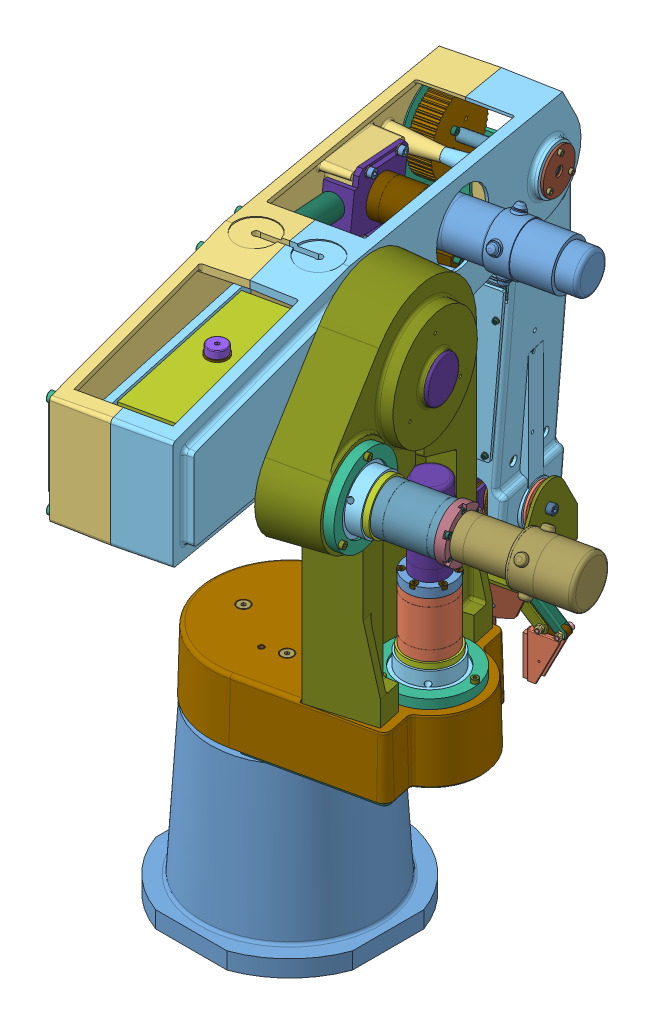
SolidWorks assembly Robot_ericc, configuration Défaut. Lengths in mm.
Overall size (506.37 616.21 601.95).
349 component instances, 132 part files, 24 mates.
Components (placement in the parent):
- Ens_Socle-1: Ens_Socle [Défaut] at origin size (212.48 231.5 219.24)
  - Socle-1: Socle [Default] at origin size (212.48 180 219.24)
  - Fourreau_200-604-1: Fourreau_200-604 [Défaut] at (0 176.5 0) x (-0.083866 0 0.996477) z (-0.996477 0 -0.083866) size (96 55 96)
  - CHC-M6_20-1: CHC-M6_20 [ISO 4762 M6 x 20 --- 20C] at (3.6062 156 -42.8485) x (0 1 0) z (-0.546944 0 0.837169) size (26 10 10)
  - poulie lacet-1: poulie lacet [Défaut] at (0 206.5 0) x (0.433454 0 0.901176) z (0 1 0) size (124 124 27)
  - Rondelle M6-1: Rondelle M6 [Washer ISO 7089 - 6] at (-35.9297 209 -24.5216) x (0 -1 0) z (0 0 1) size (1.6 12 12)
  - CHC-M6_25-1: CHC-M6_25 [ISO 4762 M6 x 25 --- 25C] at (-35.9297 216.6 -24.5216) x (0 -1 0) z (0.040163 0 0.999193) size (31 10 10)
  - Couvercle_300-732-1: Couvercle_300-732 [Défaut] at (0 175.5 0) x (-0.570868 0 0.821042) z (-0.821042 0 -0.570868) size (65 10.5 65)
  - CHC-M4_16-1: CHC-M4_16 [ISO 4762 M4 x 16 --- 16C] at (25.3374 166.5 -11.917) x (0 1 0) z (-0.937005 0 0.349316) size (20 7 7)
  - CHC-M4_16-2: CHC-M4_16 [ISO 4762 M4 x 16 --- 16C] at (-22.9892 166.5 -15.9843) x (0 1 0) z (0.771019 0 0.636812) size (20 7 7)
  - CHC-M4_16-3: CHC-M4_16 [ISO 4762 M4 x 16 --- 16C] at (-2.3482 166.5 27.9014) x (0 1 0) z (0.165986 0 -0.986128) size (20 7 7)
  - CHC-M6_25-2: CHC-M6_25 [ISO 4762 M6 x 25 --- 25C] at (-3.2715 216.6 43.3768) x (0 -1 0) z (0.845245 0 -0.534379) size (31 10 10)
  - CHC-M6_25-3: CHC-M6_25 [ISO 4762 M6 x 25 --- 25C] at (39.2011 216.6 -18.8552) x (0 -1 0) z (-0.885408 0 -0.464814) size (31 10 10)
  - Rondelle M6-2: Rondelle M6 [Washer ISO 7089 - 6] at (-3.2715 209 43.3768) x (0 -1 0) z (0.866025 0 -0.5) size (1.6 12 12)
  - Rondelle M6-3: Rondelle M6 [Washer ISO 7089 - 6] at (39.2011 209 -18.8552) x (0 -1 0) z (-0.866025 0 -0.5) size (1.6 12 12)
  - CHC-M6_20-2: CHC-M6_20 [ISO 4762 M6 x 20 --- 20C] at (-38.911 156 18.3012) x (0 1 0) z (0.998482 0 0.055083) size (26 10 10)
  - CHC-M6_20-3: CHC-M6_20 [ISO 4762 M6 x 20 --- 20C] at (35.3048 156 24.5473) x (0 1 0) z (-0.451538 0 -0.892252) size (26 10 10)
- SE_Chaise-1: SE_Chaise [Défaut] at (0 253.5 0) x (-0.212271 0 -0.977211) z (0 -1 0) size (256.43 420.65 448.71)
  - SE-Assise-1: SE-Assise [Défaut] at origin size (171.51 268.51 86)
    - Assise_100-032-1: Assise_100-032 [Default] at origin size (171.51 268.51 67)
    - Axe_200-464-1: Axe_200-464 [Défaut] at (0 0 11.5) x (0 0 1) z (1 0 0) size (76 96 96)
    - Goupille Çlastique , 6x20-1: Goupille Çlastique , 6x20 [Défaut] at (-40 0 10) x (1 0 0) z (0 -1 0) size (5.98 20 6)
    - Goupille Çlastique , 6x20-2: Goupille Çlastique , 6x20 [Défaut] at (40 0 10) x (1 0 0) z (0 -1 0) size (5.98 20 6)
    - visFHC M6-16-1: visFHC M6-16 [B18.3.5M - 6 x 1.0 x 16 Socket FCHS  -- 16S] at (0 -42 0) x (0 0 1) z (-1 0 0) size (16 11.7 11.7)
    - visFHC M6-16-2: visFHC M6-16 [B18.3.5M - 6 x 1.0 x 16 Socket FCHS  -- 16S] at (-36.3731 21 0) x (0 0 1) z (0.5 0.866025 0) size (16 11.7 11.7)
    - visFHC M6-16-3: visFHC M6-16 [B18.3.5M - 6 x 1.0 x 16 Socket FCHS  -- 16S] at (36.3731 21 0) x (0 0 1) z (0.5 -0.866025 0) size (16 11.7 11.7)
    - SKF_7204-1: SKF_7204 [SKF - 7204 BE - 10,DE,NC,10_68] at (0 0 31) x (0 0 1) z (-1 0 0) size (14 47 47)
    - SKF_7204-2: SKF_7204 [SKF - 7204 BE - 10,DE,NC,10_68] at (0 0 67.5) x (0 0 -1) z (1 0 0) size (14 47 47)
    - Entrtoise_200-006-1: Entrtoise_200-006 [Default] at (0 0 38) x (1 0 0) z (0 -1 0) size (47 22.5 47)
    - Capot_201-294-1: Capot_201-294 [Défaut] at (0 0.5 67) size (170 180.5 2)
  - Dossier-1: Dossier [Défaut] at (-0.0064 64.9972 -279) x (1 0 0) z (0 1 0) size (234.27 388.58 71.5)
  - Moto-rÇducteur lacet-1: Moto-rÇducteur lacet [Défaut] at (2.5917 125.4972 -183.1) x (0 0 -1) z (0.5 0.866025 0) size (236.28 90 90)
    - Corps moto-rÇducteur-1: Corps moto-rÇducteur [Default] at origin size (199.6 50 51)
      - Moteur Parvex RS120G-1: Moteur Parvex RS120G [Défaut] at origin size (126 39.96 39.96)
      - Vis CHC M4x10-1: Vis CHC M4x10 [Défaut] at (-91.1 0 22) x (0 0 1) z (-1 0 0) size (7 7 14)
      - Entretoise-m-r-1: Entretoise-m-r [Défaut] at (-92.6 0 0) size (59.8 50 50)
      - RÇducteur Harmonic Drive HDUC 14 1U-CC-1: RÇducteur Harmonic Drive HDUC 14 1U-CC [Défaut] at (-92.6 0 0) size (123.2 50 50)
      - Vis CHC M4x10-2: Vis CHC M4x10 [Défaut] at (-91.1 -19.0526 11) x (0 -0.866025 0.5) z (-1 0 0) size (7 7 14)
      - Vis CHC M4x10-3: Vis CHC M4x10 [Défaut] at (-91.1 -19.0526 -11) x (0 -0.866025 -0.5) z (-1 0 0) size (7 7 14)
      - Vis CHC M4x10-4: Vis CHC M4x10 [Défaut] at (-91.1 0 -22) x (0 0 -1) z (-1 0 0) size (7 7 14)
      - Vis CHC M4x10-5: Vis CHC M4x10 [Défaut] at (-91.1 19.0526 -11) x (0 0.866025 -0.5) z (-1 0 0) size (7 7 14)
      - Vis CHC M4x10-6: Vis CHC M4x10 [Défaut] at (-91.1 19.0526 11) x (0 0.866025 0.5) z (-1 0 0) size (7 7 14)
      - Vis CHC M4-6-1: Vis CHC M4-6 [Défaut] at (-90.1 9.8995 9.8995) x (0 0 -1) z (1 0 0) size (6 6 10)
      - Vis CHC M4-6-2: Vis CHC M4-6 [Défaut] at (-90.1 -9.8995 9.8995) x (0 1 0) z (1 0 0) size (6 6 10)
      - Vis CHC M4-6-3: Vis CHC M4-6 [Défaut] at (-90.1 -9.8995 -9.8995) x (0 0 1) z (1 0 0) size (6 6 10)
      - Vis CHC M4-6-4: Vis CHC M4-6 [Défaut] at (-90.1 9.8995 -9.8995) x (0 -1 0) z (1 0 0) size (6 6 10)
      - Arbre de sortie-1: Arbre de sortie [Défaut] at (-159.6 0 0) size (40 8 8)
    - Palier-1: Palier [Défaut] at (-162.6 0 0) size (88.18 90 90)
      - Porte poulie motrice-1: Porte poulie motrice [Défaut] at origin size (73.68 74 74)
      - Bride-1: Bride [Défaut] at (-22.5 3 0) x (0 0 -1) z (-1 0 0) size (90 90 10)
      - Flasque-1: Flasque [Défaut] at (6 0 0) x (0 -0.664186 0.747567) z (-1 0 0) size (54 54 6)
      - VisCHC M4-40-1: VisCHC M4-40 [Défaut] at (-36 -16.2635 16.2635) x (0 0.997296 -0.073485) z (1 0 0) size (7 7 44)
      - VisCHC M4-40-2: VisCHC M4-40 [Défaut] at (-36 16.2635 16.2635) x (0 -0.073485 -0.997296) z (1 0 0) size (7 7 44)
      - VisCHC M4-40-3: VisCHC M4-40 [Défaut] at (-36 16.2635 -16.2635) x (0 -0.997296 0.073485) z (1 0 0) size (7 7 44)
      - VisCHC M4-40-4: VisCHC M4-40 [Défaut] at (-36 -16.2635 -16.2635) x (0 0.073485 0.997296) z (1 0 0) size (7 7 44)
      - anneau Çlastique int d32-1: anneau Çlastique int d32 [Défaut] at (-48.6 0 0) x (0 0 1) z (-1 0 0) size (33.7 32.99 1.2)
      - Vis CHC M4x10-1: Vis CHC M4x10 [Défaut] at (4.5 20 0) x (0 0 -1) z (1 0 0) size (7 7 14)
      - Vis CHC M4x10-2: Vis CHC M4x10 [Défaut] at (4.5 10 17.3205) x (0 0.866025 -0.5) z (1 0 0) size (7 7 14)
      - Vis CHC M4x10-3: Vis CHC M4x10 [Défaut] at (4.5 -10 17.3205) x (0 0.866025 0.5) z (1 0 0) size (7 7 14)
      - Vis CHC M4x10-4: Vis CHC M4x10 [Défaut] at (4.5 -20 0) x (0 0 1) z (1 0 0) size (7 7 14)
      - Vis CHC M4x10-5: Vis CHC M4x10 [Défaut] at (4.5 -10 -17.3205) x (0 -0.866025 0.5) z (1 0 0) size (7 7 14)
      - Vis CHC M4x10-6: Vis CHC M4x10 [Défaut] at (4.5 10 -17.3205) x (0 -0.866025 -0.5) z (1 0 0) size (7 7 14)
    - SKF 6002-1: SKF 6002 [SKF - 6002 - 12,DE,NC,12_68] at (-206.7 0 0) size (9 32 32)
    - SKF 6002-2: SKF 6002 [SKF - 6002 - 12,DE,NC,12_68] at (-185.6 0 0) size (9 32 32)
  - vis CHC M6-25-1: vis CHC M6-25 [ISO 4762 M6 x 25 --- 25S] at (-57.0064 122.9972 16) x (0 0 -1) z (-0.036606 -0.99933 0) size (31 10 10)
  - vis CHC M6-25-2: vis CHC M6-25 [ISO 4762 M6 x 25 --- 25S] at (-57.0064 77.9972 16) x (0 0 -1) z (-0.036606 -0.99933 0) size (31 10 10)
  - vis CHC M6-25-3: vis CHC M6-25 [ISO 4762 M6 x 25 --- 25S] at (56.9936 122.9972 16) x (0 0 -1) z (-0.036606 -0.99933 0) size (31 10 10)
  - vis CHC M6-25-4: vis CHC M6-25 [ISO 4762 M6 x 25 --- 25S] at (56.9936 77.9972 16) x (0 0 -1) z (-0.036606 -0.99933 0) size (31 10 10)
  - Goupille Çlastique , 6x20-1: Goupille Çlastique , 6x20 [Défaut] at (66.9936 122.9972 2) x (1 0 0) z (0 -1 0) size (5.98 20 6)
  - Goupille Çlastique , 6x20-2: Goupille Çlastique , 6x20 [Défaut] at (-42.0064 77.9972 2) x (1 0 0) z (0 -1 0) size (5.98 20 6)
  - Moteur Epaule-1: Moteur Epaule [Défaut] at (-95.2692 334.8972 -221) x (0 1 0) z (0.162984 0 0.986629) size (264.08 126.67 126.67)
    - Moteur RS210-1: Moteur RS210 [Défaut] at origin size (135.4 52 52)
    - entretoise-m-r bras-1: entretoise-m-r bras [Défaut] at (-120.4 0 0) x (1 0 0) z (0 0.162984 0.986629) size (59.8 54 54)
    - RÇducteur Harmonic Drive bras-1: RÇducteur Harmonic Drive bras [Défaut] at (-120.4 0 0) x (1 0 0) z (0 0.634463 0.772953) size (123.2 51.79 50)
    - Vis CHC M4x10-1: Vis CHC M4x10 [Défaut] at (-117.9 11.3806 8.1537) x (0 0.924309 0.381646) z (1 0 0) size (7 7 14)
    - Vis CHC M4x10-2: Vis CHC M4x10 [Défaut] at (-117.9 -8.1537 11.3806) x (0 -0.381646 0.924309) z (1 0 0) size (7 7 14)
    - Vis CHC M4x10-3: Vis CHC M4x10 [Défaut] at (-117.9 -11.3806 -8.1537) x (0 -0.924309 -0.381646) z (1 0 0) size (7 7 14)
    - Vis CHC M4x10-4: Vis CHC M4x10 [Défaut] at (-117.9 8.1537 -11.3806) x (0 0.381646 -0.924309) z (1 0 0) size (7 7 14)
    - Vis CHC M3-10-1: Vis CHC M3-10 [Défaut] at (-118.9 3.5857 21.7058) x (0 -0.692088 -0.721813) z (-1 0 0) size (5.5 5.5 13)
    - Vis CHC M3-10-2: Vis CHC M3-10 [Défaut] at (-118.9 -17.005 13.9582) x (0 0.279064 -0.960272) z (-1 0 0) size (5.5 5.5 13)
    - Vis CHC M3-10-3: Vis CHC M3-10 [Défaut] at (-118.9 -20.5906 -7.7476) x (0 0.971152 -0.238459) z (-1 0 0) size (5.5 5.5 13)
    - Vis CHC M3-10-4: Vis CHC M3-10 [Défaut] at (-118.9 -3.5857 -21.7058) x (0 0.692088 0.721813) z (-1 0 0) size (5.5 5.5 13)
    - Vis CHC M3-10-5: Vis CHC M3-10 [Défaut] at (-118.9 17.005 -13.9582) x (0 -0.279064 0.960272) z (-1 0 0) size (5.5 5.5 13)
    - Vis CHC M3-10-6: Vis CHC M3-10 [Défaut] at (-118.9 20.5906 7.7476) x (0 -0.971152 0.238459) z (-1 0 0) size (5.5 5.5 13)
    - Palier-1: Palier [Défaut] at (-190.4 0 0) x (1 0 0) z (0 0.634463 0.772953) size (88.18 90 90)
      - Porte poulie motrice-1: Porte poulie motrice [Défaut] at origin size (73.68 74 74)
      - Bride-1: Bride [Défaut] at (-22.5 3 0) x (0 0 -1) z (-1 0 0) size (90 90 10)
      - Flasque-1: Flasque [Défaut] at (6 0 0) x (0 -0.664186 0.747567) z (-1 0 0) size (54 54 6)
      - VisCHC M4-40-1: VisCHC M4-40 [Défaut] at (-36 -16.2635 16.2635) x (0 0.997296 -0.073485) z (1 0 0) size (7 7 44)
      - VisCHC M4-40-2: VisCHC M4-40 [Défaut] at (-36 16.2635 16.2635) x (0 -0.073485 -0.997296) z (1 0 0) size (7 7 44)
      - VisCHC M4-40-3: VisCHC M4-40 [Défaut] at (-36 16.2635 -16.2635) x (0 -0.997296 0.073485) z (1 0 0) size (7 7 44)
      - VisCHC M4-40-4: VisCHC M4-40 [Défaut] at (-36 -16.2635 -16.2635) x (0 0.073485 0.997296) z (1 0 0) size (7 7 44)
      - anneau Çlastique int d32-1: anneau Çlastique int d32 [Défaut] at (-48.6 0 0) x (0 0 1) z (-1 0 0) size (33.7 32.99 1.2)
      - Vis CHC M4x10-1: Vis CHC M4x10 [Défaut] at (4.5 20 0) x (0 0 -1) z (1 0 0) size (7 7 14)
      - Vis CHC M4x10-2: Vis CHC M4x10 [Défaut] at (4.5 10 17.3205) x (0 0.866025 -0.5) z (1 0 0) size (7 7 14)
      - Vis CHC M4x10-3: Vis CHC M4x10 [Défaut] at (4.5 -10 17.3205) x (0 0.866025 0.5) z (1 0 0) size (7 7 14)
      - Vis CHC M4x10-4: Vis CHC M4x10 [Défaut] at (4.5 -20 0) x (0 0 1) z (1 0 0) size (7 7 14)
      - Vis CHC M4x10-5: Vis CHC M4x10 [Défaut] at (4.5 -10 -17.3205) x (0 -0.866025 0.5) z (1 0 0) size (7 7 14)
      - Vis CHC M4x10-6: Vis CHC M4x10 [Défaut] at (4.5 10 -17.3205) x (0 -0.866025 -0.5) z (1 0 0) size (7 7 14)
    - SKF 6002-1: SKF 6002 [SKF - 6002 - 12,DE,NC,12_68] at (-213.4 0 0) size (9 32 32)
    - SKF 6002-2: SKF 6002 [SKF - 6002 - 12,DE,NC,12_68] at (-234.5 0 0) size (9 32 32)
  - Vis_CHC_M4-16-1: Vis_CHC_M4-16 [ISO 4762 M4 x 12 --- 12C] at (-133.3743 135.9972 -202) x (0 -1 0) z (0 0 1) size (20 7 7)
  - Vis_CHC_M4-16-2: Vis_CHC_M4-16 [ISO 4762 M4 x 12 --- 12C] at (-0.0064 167.9972 -12) x (0 0 1) z (0 1 0) size (20 7 7)
  - Vis_CHC_M4-16-3: Vis_CHC_M4-16 [ISO 4762 M4 x 12 --- 12C] at (-35.5134 106.4972 -12) x (0 0 1) z (-0.866025 -0.5 0) size (20 7 7)
  - Vis_CHC_M4-16-4: Vis_CHC_M4-16 [ISO 4762 M4 x 12 --- 12C] at (35.5007 106.4972 -12) x (0 0 1) z (0.866025 -0.5 0) size (20 7 7)
  - Vis_CHC_M4-16-5: Vis_CHC_M4-16 [ISO 4762 M4 x 12 --- 12C] at (-97.8672 135.9972 -263.5) x (0 -1 0) z (-0.866025 0 -0.5) size (20 7 7)
  - Vis_CHC_M4-16-6: Vis_CHC_M4-16 [ISO 4762 M4 x 12 --- 12C] at (-62.3602 135.9972 -202) x (0 -1 0) z (0.866025 0 -0.5) size (20 7 7)
  - Bouchon-1: Bouchon [Défaut] at (-0.0064 133.9972 -279) size (46 5.5 46)
  - Couvercle_301-396-1: Couvercle_301-396 [Défaut] at (-0.0064 71.9972 -279) x (0.866025 0 0.5) z (-0.5 0 0.866025) size (66 8 66)
  - Vis_CHC_M4-16-7: Vis_CHC_M4-16 [ISO 4762 M4 x 12 --- 12C] at (-0.0064 71.9972 -307.5) x (0 1 0) z (-0.976883 0 -0.213777) size (20 7 7)
  - Vis_CHC_M4-16-8: Vis_CHC_M4-16 [ISO 4762 M4 x 12 --- 12C] at (-24.6881 71.9972 -264.75) x (0 1 0) z (0.303305 0 0.952894) size (20 7 7)
  - Vis_CHC_M4-16-9: Vis_CHC_M4-16 [ISO 4762 M4 x 12 --- 12C] at (24.6754 71.9972 -264.75) x (0 1 0) z (0.673578 0 -0.739117) size (20 7 7)
  - Ecrou Ö encoches, M 17-1: Ecrou Ö encoches, M 17 [Défaut] at (0 0 75.5) x (-0.99693 -0.078302 0) z (-0.078302 0.99693 0) size (27.71 5 27.71)
  - Rondelle frein de 17-1: Rondelle frein de 17 [Défaut] at (0 0 74.5) x (-0.99693 -0.078302 0) z (-0.078302 0.99693 0) size (33.42 5.39 32.18)
- Bras-1: Bras [Défaut] at (-0.5391 505.7717 6.953) x (0.212271 0 0.977211) z (-0.977211 0 0.212271) size (576.57 148.84 242.4)
  - BrasDroit-2: BrasDroit [Défaut] at origin size (576.57 148.84 66)
  - GoupillePosition-1: GoupillePosition [Défaut] at (-30.6737 92.2283 0) x (0 0 1) z (-1 0 0) size (10 8 8)
  - GoupillePosition-3: GoupillePosition [Défaut] at (234.3263 -27.2717 0) x (0 0 1) z (-1 0 0) size (10 8 8)
  - GoupillePosition-4: GoupillePosition [Défaut] at (-227.6737 51.7283 0) x (0 0 1) z (-1 0 0) size (10 8 8)
  - BrasGauche-2: BrasGauche [Défaut] at (-6.6737 26.7283 0) size (576.57 148.84 101.36)
  - Vis C HC, M 6x70-1: Vis C HC, M 6x70 [Défaut] at (-227.6737 51.7283 55) x (-0.629032 0.777379 0) z (0.777379 0.629032 0) size (10 76 10)
  - Vis C HC, M 6x70-7: Vis C HC, M 6x70 [Défaut] at (-30.6737 92.2283 55) x (0.427468 -0.90403 0) z (-0.90403 -0.427468 0) size (10 76 10)
  - Vis C HC, M 6x70-9: Vis C HC, M 6x70 [Défaut] at (234.3263 -27.2717 55) x (0.427468 -0.90403 0) z (-0.90403 -0.427468 0) size (10 76 10)
  - Vis C HC, M 6x70-11: Vis C HC, M 6x70 [Défaut] at (-165.6737 -17.2717 55) x (0.427468 -0.90403 0) z (-0.90403 -0.427468 0) size (10 76 10)
  - Vis C HC, M 6x70-15: Vis C HC, M 6x70 [Défaut] at (234.3263 77.7283 55) x (0.427468 -0.90403 0) z (-0.90403 -0.427468 0) size (10 76 10)
  - Vis C HC, M 6x70-21: Vis C HC, M 6x70 [Défaut] at (23.3263 91.126 55) x (0.427468 -0.90403 0) z (-0.90403 -0.427468 0) size (10 76 10)
  - Vis C HC, M 6x70-23: Vis C HC, M 6x70 [Défaut] at (-6.6737 -38.7717 55) x (0.427468 -0.90403 0) z (-0.90403 -0.427468 0) size (10 76 10)
  - contre_poids-1: contre_poids [Défaut] at (123.9539 42.7283 -46) size (175 60 60)
  - Vis C HC, M 8x70-1: Vis C HC, M 8x70 [Défaut] at (117.4539 78.7283 -16) x (0.870431 0 -0.492291) z (0.492291 0 0.870431) size (20 78.34 20)
  - Rondelle L, 8-1: Rondelle L, 8 [Défaut] at (117.4539 75.7283 -16) size (22 1.5 22)
  - Rondelle L, 8-3: Rondelle L, 8 [Défaut] at (117.4539 77.2283 -16) size (22 1.5 22)
  - SKF_6001-1: SKF_6001 [SKF - 6001 - 10,DE,NC,10_68] at (-286.6737 26.7283 -58) x (0 0 -1) z (1 0 0) size (8 28 28)
  - Couvercle_M300-013-1: Couvercle_M300-013 [Défaut] at (-286.6737 26.7283 -64) x (0 0 1) z (-1 0 0) size (4.5 45 45)
  - CHC_M3-10-1: CHC_M3-10 [ISO 4762 M3 x 10 --- 10C] at (-302.2622 17.7283 -69.5) x (0 0 1) z (-1 0 0) size (13 5.5 5.5)
  - CHC_M3-10-3: CHC_M3-10 [ISO 4762 M3 x 10 --- 10C] at (-286.6737 44.7283 -69.5) x (0 0 1) z (-1 0 0) size (13 5.5 5.5)
  - CHC_M3-10-9: CHC_M3-10 [ISO 4762 M3 x 10 --- 10C] at (-271.0852 17.7283 -69.5) x (0 0 1) z (-1 0 0) size (13 5.5 5.5)
  - Verin-pince-1: Verin-pince [Défaut] at (-48.6737 7.2342 -0.5445) x (-1 0 0) z (0 -0.130938 0.991391) size (269.69 47.71 50)
    - Support-verin-1: Support-verin [Défaut] at origin size (170 44 50)
    - 5079 DSN-25-80-1: 5079 DSN-25-80 [Défaut] at (-118.1875 36.1693 13.898) x (0 -0.972057 -0.234746) z (1 0 0) size (36.95 32 205.57)
      - Corps-1: Corps [Défaut] at (13.1476 11.1224 0) size (27 27 173.5)
      - Piston-1: Piston [Défaut] at (13.1476 11.1224 4.0685) size (25 25 177.5)
      - Ecrou-1: Ecrou [Défaut] at (13.1476 11.1224 2.0036) size (36.95 32 11)
  - CHC_M3-10-10: CHC_M3-10 [ISO 4762 M3 x 10 --- 10C] at (106.3263 -1.975 9.6121) x (0 0.991391 0.130938) z (0 -0.130938 0.991391) size (13 5.5 5.5)
  - CHC_M3-10-11: CHC_M3-10 [ISO 4762 M3 x 10 --- 10C] at (106.3263 0.8402 -11.7028) x (0 0.991391 0.130938) z (-0.130938 -0.129811 0.982855) size (13 5.5 5.5)
  - SupportMoteur_M300-005-1: SupportMoteur_M300-005 [Défaut] at (-166.3149 43.5192 23.5) x (-0.988512 -0.151141 0) z (0 0 -1) size (75 70 28)
  - Rondelle Z, 3-1: Rondelle Z, 3 [Défaut] at (106.3263 0.9992 10.0049) x (1 0 0) z (0 -0.130938 0.991391) size (6 0.8 6)
  - Rondelle Z, 3-3: Rondelle Z, 3 [Défaut] at (106.3263 3.8144 -11.31) x (1 0 0) z (0 -0.130938 0.991391) size (6 0.8 6)
  - VisCHC_M5-16-1: VisCHC_M5-16 [ISO 4762 M5 x 16 --- 16C] at (-149.3329 75.8068 12.5) x (0 0 1) z (-0.747365 -0.664413 0) size (21 8.5 8.5)
  - VisCHC_M5-16-3: VisCHC_M5-16 [ISO 4762 M5 x 16 --- 16C] at (-141.3413 15.8945 12.5) x (0 0 1) z (-1 0 0) size (21 8.5 8.5)
  - VisCHC_M5-16-5: VisCHC_M5-16 [ISO 4762 M5 x 16 --- 16C] at (-185.0651 10.9723 12.5) x (0 0 1) z (-1 0 0) size (21 8.5 8.5)
  - VisCHC_M5-16-7: VisCHC_M5-16 [ISO 4762 M5 x 16 --- 16C] at (-193.005 70.4446 12.5) x (0 0 1) z (-1 0 0) size (21 8.5 8.5)
  - Rondelle Z, 5-1: Rondelle Z, 5 [Défaut] at (-185.0651 10.9723 18.5) x (1 0 0) z (0 1 0) size (10 1 10)
  - Rondelle Z, 5-3: Rondelle Z, 5 [Défaut] at (-193.005 70.4446 18.5) x (1 0 0) z (0 1 0) size (10 1 10)
  - Rondelle Z, 5-5: Rondelle Z, 5 [Défaut] at (-149.3329 75.8068 18.5) x (1 0 0) z (0 1 0) size (10 1 10)
  - Rondelle Z, 5-7: Rondelle Z, 5 [Défaut] at (-141.3413 15.8945 18.5) x (1 0 0) z (0 1 0) size (10 1 10)
  - AXE_Bras-1: AXE_Bras [Défaut] at (-6.6737 26.7283 -80) x (0 0 -1) z (-1 0 0) size (72.5 126.04 126.04)
    - AXE_M300-010-1: AXE_M300-010 [Défaut] at origin size (72.5 98 98)
    - Poulie_M300-014-1: Poulie_M300-014 [Défaut] at (-4 0 0) size (30 126.04 126.04)
    - Vic_CHCM6-16-1: Vic_CHCM6-16 [ISO 4762 M6 x 16 --- 16C] at (9.2 22 -38.1051) x (-1 0 0) z (0 0.831566 -0.555426) size (22 10 10)
    - Goupille6-32-1: Goupille6-32 [Parallel Pin ISO 8734 - 6 x 32 - A - St] at (-14 44 0) size (32 6 6)
    - Goupille6-32-2: Goupille6-32 [Parallel Pin ISO 8734 - 6 x 32 - A - St] at (-14 -31.1127 31.1127) x (1 0 0) z (0 -0.90193 0.431882) size (32 6 6)
    - EntretoiseM200-006-1: EntretoiseM200-006 [Défaut] at (35.5 0 0) x (1 0 0) z (0 -0.984877 -0.173252) size (21.5 47 47)
    - 7204_Rlt-Billes-1: 7204_Rlt-Billes [SKF - 7204 BE - 10,DE,NC,10_68] at (7 0 0) x (1 0 0) z (0 -0.825996 0.563676) size (14 47 47)
    - 7204_Rlt-Billes-2: 7204_Rlt-Billes [SKF - 7204 BE - 10,DE,NC,10_68] at (42.5 0 0) x (-1 0 0) z (0 -0.662732 0.748856) size (14 47 47)
    - Ecrou Ö encoches, M 20-1: Ecrou Ö encoches, M 20 [Défaut] at (50.5 0 0) x (0 0.493503 -0.869744) z (0 -0.869744 -0.493503) size (31.75 7.06 31.75)
    - Rondelle frein de 20-1: Rondelle frein de 20 [Défaut] at (49.5 0 0) x (0 0.317084 0.948397) z (0 0.948397 -0.317084) size (36.64 6.14 35.22)
    - Rondelle M, 6-1: Rondelle M, 6 [Défaut] at (2 22 -38.1051) x (0 -0.99765 -0.068521) z (0 -0.068521 0.99765) size (14 1.2 14)
    - Vic_CHCM6-16-2: Vic_CHCM6-16 [ISO 4762 M6 x 16 --- 16C] at (9.2 -44 0) x (-1 0 0) z (0 -0.896796 -0.442445) size (22 10 10)
    - Vic_CHCM6-16-3: Vic_CHCM6-16 [ISO 4762 M6 x 16 --- 16C] at (9.2 22 38.1051) x (-1 0 0) z (0 0.06523 0.99787) size (22 10 10)
    - Rondelle M, 6-2: Rondelle M, 6 [Défaut] at (2 -44 0) x (0 0.439484 0.89825) z (0 0.89825 -0.439484) size (14 1.2 14)
    - Rondelle M, 6-3: Rondelle M, 6 [Défaut] at (2 22 38.1051) x (0 0.558165 -0.82973) z (0 -0.82973 -0.558165) size (14 1.2 14)
  - Rondelle M, 6-1: Rondelle M, 6 [Défaut] at (-6.6737 -3.0038 -59) x (1 0 0) z (0 -1 0) size (14 1.2 14)
  - Rondelle M, 6-3: Rondelle M, 6 [Défaut] at (-32.4225 41.5944 -59) x (1 0 0) z (0 -1 0) size (14 1.2 14)
  - Rondelle M, 6-5: Rondelle M, 6 [Défaut] at (19.0751 41.5944 -59) x (1 0 0) z (0 -1 0) size (14 1.2 14)
  - Vic_CHCM6-16-7: Vic_CHCM6-16 [ISO 4762 M6 x 16 --- 16C] at (-32.4225 41.5944 -51.8) x (0 0 -1) z (1 0 0) size (22 10 10)
  - Vic_CHCM6-16-9: Vic_CHCM6-16 [ISO 4762 M6 x 16 --- 16C] at (-6.6737 -3.0038 -51.8) x (0 0 -1) z (1 0 0) size (22 10 10)
  - Vic_CHCM6-16-11: Vic_CHCM6-16 [ISO 4762 M6 x 16 --- 16C] at (19.0751 41.5944 -51.8) x (0 0 -1) z (-1 0 0) size (22 10 10)
  - parallel pin unhardened_iso-1: parallel pin unhardened_iso [Parallel Pin ISO 2338 - 6 m6 x 20 - St] at (-6.6737 56.7283 -73) x (0 0 1) z (0.997282 0.073675 0) size (20 6 6)
  - parallel pin unhardened_iso-3: parallel pin unhardened_iso [Parallel Pin ISO 2338 - 6 m6 x 20 - St] at (14.5395 5.5151 -73) x (0 0 1) z (0.997282 0.073675 0) size (20 6 6)
  - Couvercle_M300-013-4: Couvercle_M300-013 [Défaut] at (-286.6737 26.7283 63) x (0 0 -1) z (1 0 0) size (4.5 45 45)
  - Rondelle Çpaisse Z, 12-1: Rondelle Çpaisse Z, 12 [Défaut] at (-286.6737 26.7283 -50.5) x (0.066998 0.997753 0) z (-0.997753 0.066998 0) size (15 3.5 15)
  - SKF_6001-2: SKF_6001 [SKF - 6001 - 10,DE,NC,10_68] at (-286.6737 26.7283 57) x (0 0 -1) z (0.798379 0.602155 0) size (8 28 28)
  - Rondelle Çpaisse Z, 12-3: Rondelle Çpaisse Z, 12 [Défaut] at (-286.6737 26.7283 49.5) x (0.444076 -0.895989 0) z (-0.895989 -0.444076 0) size (15 3.5 15)
  - CHC_M3-10-14: CHC_M3-10 [ISO 4762 M3 x 10 --- 10C] at (-271.0852 17.7283 68.5) x (0 0 -1) z (1 0 0) size (13 5.5 5.5)
  - CHC_M3-10-16: CHC_M3-10 [ISO 4762 M3 x 10 --- 10C] at (-302.2622 17.7283 68.5) x (0 0 -1) z (1 0 0) size (13 5.5 5.5)
  - CHC_M3-10-18: CHC_M3-10 [ISO 4762 M3 x 10 --- 10C] at (-286.6737 44.7283 68.5) x (0 0 -1) z (1 0 0) size (13 5.5 5.5)
  - AXE 04 021 M300 011-1: AXE 04 021 M300 011 [Défaut] at (-286.6737 26.7283 -63) x (-0.545711 0.837974 0) z (0 0 1) size (12 12 125)
  - Vis Ö bille M6-40-1: Vis Ö bille M6-40 [Défaut] at (-37.2131 63.2586 37.5) x (-0.988512 -0.151141 0) z (0.079359 -0.519031 0.851063) size (106.14 36 36)
    - socket head cap screw_iso-1: socket head cap screw_iso [PreviewCfg] at origin size (104 36 36)
    - Bille-1: Bille [Défaut] at (103.5 0 0) x (-0.326721 -0.900194 0.28793) z (-0.943911 0.295385 -0.147577) size (4 4 4)
  - hex nut gradec_iso-1: hex nut gradec_iso [Hexagon Nut ISO - 4034 - M6 - N] at (-120.7445 50.4869 37.5) x (0.022844 -0.149405 -0.988512) z (0.988512 0.151141 0) size (10 11.55 6.1)
  - MotoReduc_Coude-1: MotoReduc_Coude [Défaut] at (-166.3149 43.5192 -32.5) x (0 0 -1) z (0.805857 -0.592111 0) size (233.4 63.14 63.14)
    - RÇducteur Harmonic Drive HDUC 11 1U-CC-1: RÇducteur Harmonic Drive HDUC 11 1U-CC [Défaut] at origin size (123.2 40 40)
    - Moteur Parvex RS220F-1: Moteur Parvex RS220F [Défaut] at (141.4 0 0) x (1 0 0) z (0 0.244629 0.969617) size (210.51 52 52)
    - BrideCoude-1: BrideCoude [Défaut] at (-5 0 0) size (10 52 52)
    - Sortie reduc-1: Sortie reduc [Défaut] at (-52 0 0) size (40 10 10)
  - socket head cap screw_iso-1: socket head cap screw_iso [ISO 4762 M4 x 8 --- 8N] at (-149.016 46.1642 27) x (0 0 -1) z (0.779732 0.626114 0) size (12 7 7)
  - Rondelle, W 4-1: Rondelle, W 4 [Défaut] at (-149.016 46.1642 23) x (0 -1 0) z (1 0 0) size (7.3 1.5 7.3)
  - Rondelle, W 4-2: Rondelle, W 4 [Défaut] at (-168.9599 60.8182 23) x (1 0 0) z (0 1 0) size (7.3 1.5 7.3)
  - Rondelle, W 4-3: Rondelle, W 4 [Défaut] at (-183.6139 40.8743 23) x (0 1 0) z (-1 0 0) size (7.3 1.5 7.3)
  - Rondelle, W 4-4: Rondelle, W 4 [Défaut] at (-163.67 26.2203 23) x (-1 0 0) z (0 -1 0) size (7.3 1.5 7.3)
  - socket head cap screw_iso-2: socket head cap screw_iso [ISO 4762 M4 x 8 --- 8N] at (-168.9599 60.8182 27) x (0 0 -1) z (-0.626114 0.779732 0) size (12 7 7)
  - socket head cap screw_iso-3: socket head cap screw_iso [ISO 4762 M4 x 8 --- 8N] at (-183.6139 40.8743 27) x (0 0 -1) z (-0.779732 -0.626114 0) size (12 7 7)
  - socket head cap screw_iso-4: socket head cap screw_iso [ISO 4762 M4 x 8 --- 8N] at (-163.67 26.2203 27) x (0 0 -1) z (0.626114 -0.779732 0) size (12 7 7)
